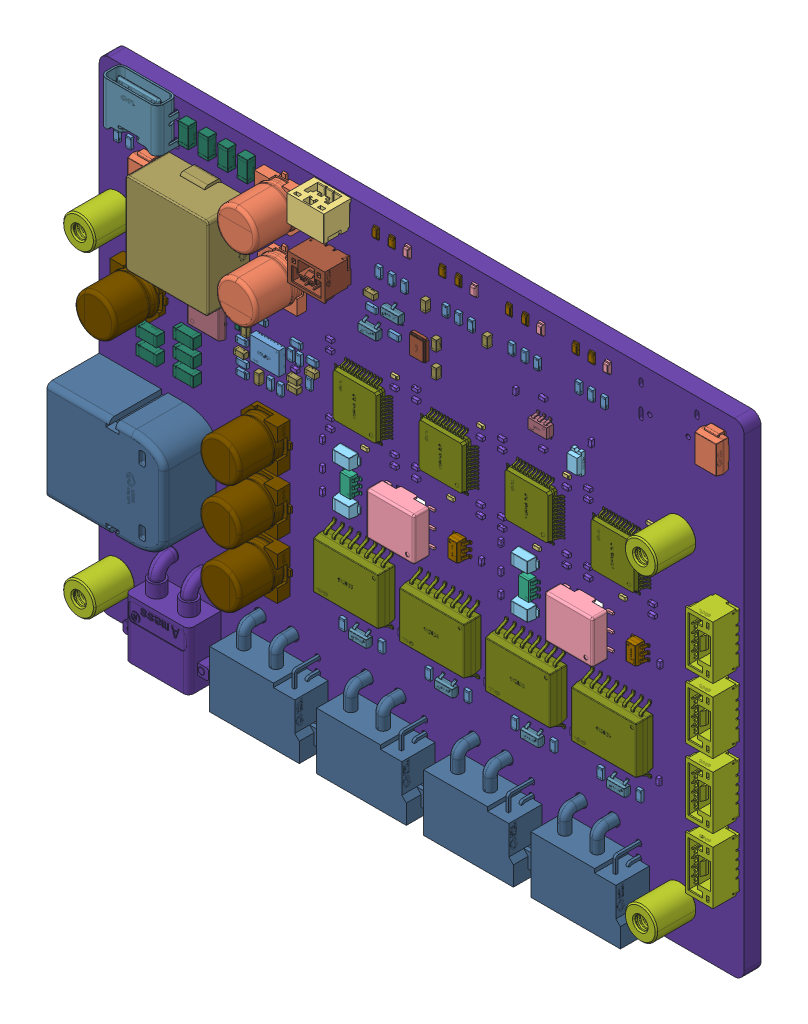
SolidWorks assembly 三合一(1), configuration 默认. Lengths in mm. (continued)
Components (placement in the parent): (continued)
- 三合一(1).step-1: 三合一(1).step [默认] at origin size (99.98 75.08 11.76) (continued)
  - X3~CRYSTAL-SMD_4P-L3.2-W2.5-BL~CRYSTAL-SMD_4P-L3.2-W2.5-BL~Huq4.step-1: X3~CRYSTAL-SMD_4P-L3.2-W2.5-BL~CRYSTAL-SMD_4P-L3.2-W2.5-BL~Huq4.step [默认] at (-11.176 22.9235 2.6301) x (0 -1 0) z (0 0 1) size (3.2 2.5 0.7)
    - CRYSTAL-SMD_4P-L3.2-W2.5-BL~CRYSTAL-SMD_4P-L3.2-W2.5-BL~nuzN.step-1: CRYSTAL-SMD_4P-L3.2-W2.5-BL~CRYSTAL-SMD_4P-L3.2-W2.5-BL~nuzN.step [默认] at origin size (3.2 2.5 0.7)
  - C143~C0603~C0603_L1.6-W0.8-H0.8~8vyH.step-1: C143~C0603~C0603_L1.6-W0.8-H0.8~8vyH.step [默认] at (-18.516 26.4431 3.0301) size (1.6 0.8 0.8)
    - C0603~C0603_L1.6-W0.8-H0.8~0uWZ.step-1: C0603~C0603_L1.6-W0.8-H0.8~0uWZ.step [默认] at origin size (1.6 0.8 0.8)
  - C141~C0603~C0603_L1.6-W0.8-H0.8~goz1.step-1: C141~C0603~C0603_L1.6-W0.8-H0.8~goz1.step [默认] at (-8.382 21.0424 3.0301) x (0 1 0) z (0 0 1) size (1.6 0.8 0.8)
    - C0603~C0603_L1.6-W0.8-H0.8~0uWZ.step-1: C0603~C0603_L1.6-W0.8-H0.8~0uWZ.step [默认] at origin size (1.6 0.8 0.8)
  - C142~C0603~C0603_L1.6-W0.8-H0.8~5pQK.step-1: C142~C0603~C0603_L1.6-W0.8-H0.8~5pQK.step [默认] at (-8.382 24.8046 3.0301) x (0 -1 0) z (0 0 1) size (1.6 0.8 0.8)
    - C0603~C0603_L1.6-W0.8-H0.8~0uWZ.step-1: C0603~C0603_L1.6-W0.8-H0.8~0uWZ.step [默认] at origin size (1.6 0.8 0.8)
  - C139~C0603~C0603_L1.6-W0.8-H0.8~dp7c.step-1: C139~C0603~C0603_L1.6-W0.8-H0.8~dp7c.step [默认] at (-10.0359 29.2101 3.0301) x (0 1 0) z (0 0 1) size (1.6 0.8 0.8)
    - C0603~C0603_L1.6-W0.8-H0.8~0uWZ.step-1: C0603~C0603_L1.6-W0.8-H0.8~0uWZ.step [默认] at origin size (1.6 0.8 0.8)
  - C140~C0603~C0603_L1.6-W0.8-H0.8~3sRw.step-1: C140~C0603~C0603_L1.6-W0.8-H0.8~3sRw.step [默认] at (-0.482 29.2101 3.0301) x (0 1 0) z (0 0 1) size (1.6 0.8 0.8)
    - C0603~C0603_L1.6-W0.8-H0.8~0uWZ.step-1: C0603~C0603_L1.6-W0.8-H0.8~0uWZ.step [默认] at origin size (1.6 0.8 0.8)
  - C3~C0402~C0603_L1.6-W0.8-H0.8~DXB2.step-1: C3~C0402~C0603_L1.6-W0.8-H0.8~DXB2.step [默认] at (-30.4075 7.8146 3.0301) x (-1 0 0) z (0 0 1) size (1.6 0.8 0.8)
    - C0603~C0603_L1.6-W0.8-H0.8~0uWZ.step-1: C0603~C0603_L1.6-W0.8-H0.8~0uWZ.step [默认] at origin size (1.6 0.8 0.8)
  - C4~C0402~C0603_L1.6-W0.8-H0.8~lKWs.step-1: C4~C0402~C0603_L1.6-W0.8-H0.8~lKWs.step [默认] at (-35.8689 6.5373 3.0301) x (0 1 0) z (0 0 1) size (1.6 0.8 0.8)
    - C0603~C0603_L1.6-W0.8-H0.8~0uWZ.step-1: C0603~C0603_L1.6-W0.8-H0.8~0uWZ.step [默认] at origin size (1.6 0.8 0.8)
  - C5~C0402~C0603_L1.6-W0.8-H0.8~kbQX.step-1: C5~C0402~C0603_L1.6-W0.8-H0.8~kbQX.step [默认] at (-30.4075 9.0339 3.0301) x (-1 0 0) z (0 0 1) size (1.6 0.8 0.8)
    - C0603~C0603_L1.6-W0.8-H0.8~0uWZ.step-1: C0603~C0603_L1.6-W0.8-H0.8~0uWZ.step [默认] at origin size (1.6 0.8 0.8)
  - C6~C0402~C0603_L1.6-W0.8-H0.8~siWF.step-1: C6~C0402~C0603_L1.6-W0.8-H0.8~siWF.step [默认] at (-27.6478 11.2673 3.0301) size (1.6 0.8 0.8)
    - C0603~C0603_L1.6-W0.8-H0.8~0uWZ.step-1: C0603~C0603_L1.6-W0.8-H0.8~0uWZ.step [默认] at origin size (1.6 0.8 0.8)
  - C7~C0402~C0603_L1.6-W0.8-H0.8~Gngn.step-1: C7~C0402~C0603_L1.6-W0.8-H0.8~Gngn.step [默认] at (-37.8461 11.938 3.0301) x (0 -1 0) z (0 0 1) size (1.6 0.8 0.8)
    - C0603~C0603_L1.6-W0.8-H0.8~0uWZ.step-1: C0603~C0603_L1.6-W0.8-H0.8~0uWZ.step [默认] at origin size (1.6 0.8 0.8)
  - C8~C0402~C0603_L1.6-W0.8-H0.8~xPmg.step-1: C8~C0402~C0603_L1.6-W0.8-H0.8~xPmg.step [默认] at (-47.1845 12.2066 -0.4) x (0 1 0) z (0 0 -1) size (1.6 0.8 0.8)
    - C0603~C0603_L1.6-W0.8-H0.8~0uWZ.step-1: C0603~C0603_L1.6-W0.8-H0.8~0uWZ.step [默认] at origin size (1.6 0.8 0.8)
  - C9~C0402~C0603_L1.6-W0.8-H0.8~Sl4T.step-1: C9~C0402~C0603_L1.6-W0.8-H0.8~Sl4T.step [默认] at (-38.6381 8.4432 3.0301) size (1.6 0.8 0.8)
    - C0603~C0603_L1.6-W0.8-H0.8~0uWZ.step-1: C0603~C0603_L1.6-W0.8-H0.8~0uWZ.step [默认] at origin size (1.6 0.8 0.8)
  - U117~SOT-23-5_L2.9-W1.6-P0.95-LS2.8-BL~SOT-23-5_L2.9-W1.6-P0.95-LS2.8-BL~xtDB.step-1: U117~SOT-23-5_L2.9-W1.6-P0.95-LS2.8-BL~SOT-23-5_L2.9-W1.6-P0.95-LS2.8-BL~xtDB.step [默认] at (8.032 21.986 3.3801) x (-1 0 0) z (0 0 1) size (2.92 2.8 1.15)
    - SOT-23-5_L2.9-W1.6-P0.95-LS2.8-BL~SOT-23-5_L2.9-W1.6-P0.95-LS2.8-BL~GdKc.step-1: SOT-23-5_L2.9-W1.6-P0.95-LS2.8-BL~SOT-23-5_L2.9-W1.6-P0.95-LS2.8-BL~GdKc.step [默认] at origin size (2.92 2.8 1.15)
  - Q3~SOT-23-3_L2.9-W1.3-P1.90-LS2.4-BR~SOT-23-3P_L2.9-W1.3-H1.0-LS2.4-P0.95~UPIG.step-1: Q3~SOT-23-3_L2.9-W1.3-P1.90-LS2.4-BR~SOT-23-3P_L2.9-W1.3-H1.0-LS2.4-P0.95~UPIG.step [默认] at (-18.516 21.6171 2.5794) x (0 -1 0) z (0 0 1) size (2.5 2.89 1.05)
    - SOT-23-3_L2.9-W1.3-P1.90-LS2.4-BR~SOT-23-3P_L2.9-W1.3-H1.0-LS2.4-P0.95~rVWb.step-1: SOT-23-3_L2.9-W1.3-P1.90-LS2.4-BR~SOT-23-3P_L2.9-W1.3-H1.0-LS2.4-P0.95~rVWb.step [默认] at origin size (2.5 2.89 1.05)
  - D11~SOT-23-3_L2.9-W1.3-P1.90-LS2.4-BR~SOT-23-3P_L2.9-W1.3-H1.0-LS2.4-P0.95~v811.step-1: D11~SOT-23-3_L2.9-W1.3-P1.90-LS2.4-BR~SOT-23-3P_L2.9-W1.3-H1.0-LS2.4-P0.95~v811.step [默认] at (-20 -20.3843 2.5794) x (0 -1 0) z (0 0 1) size (2.5 2.89 1.05)
    - SOT-23-3_L2.9-W1.3-P1.90-LS2.4-BR~SOT-23-3P_L2.9-W1.3-H1.0-LS2.4-P0.95~rVWb.step-1: SOT-23-3_L2.9-W1.3-P1.90-LS2.4-BR~SOT-23-3P_L2.9-W1.3-H1.0-LS2.4-P0.95~rVWb.step [默认] at origin size (2.5 2.89 1.05)
  - Q4~SOT-23-3_L2.9-W1.3-P1.90-LS2.4-BR~SOT-23-3P_L2.9-W1.3-H1.0-LS2.4-P0.95~4c30.step-1: Q4~SOT-23-3_L2.9-W1.3-P1.90-LS2.4-BR~SOT-23-3P_L2.9-W1.3-H1.0-LS2.4-P0.95~4c30.step [默认] at (-15.016 25.527 2.5794) x (0 1 0) z (0 0 1) size (2.5 2.89 1.05)
    - SOT-23-3_L2.9-W1.3-P1.90-LS2.4-BR~SOT-23-3P_L2.9-W1.3-H1.0-LS2.4-P0.95~rVWb.step-1: SOT-23-3_L2.9-W1.3-P1.90-LS2.4-BR~SOT-23-3P_L2.9-W1.3-H1.0-LS2.4-P0.95~rVWb.step [默认] at origin size (2.5 2.89 1.05)
  - D12~SOT-23-3_L2.9-W1.3-P1.90-LS2.4-BR~SOT-23-3P_L2.9-W1.3-H1.0-LS2.4-P0.95~vKNW.step-1: D12~SOT-23-3_L2.9-W1.3-P1.90-LS2.4-BR~SOT-23-3P_L2.9-W1.3-H1.0-LS2.4-P0.95~vKNW.step [默认] at (-6.6667 -20.3843 2.5794) x (0 -1 0) z (0 0 1) size (2.5 2.89 1.05)
    - SOT-23-3_L2.9-W1.3-P1.90-LS2.4-BR~SOT-23-3P_L2.9-W1.3-H1.0-LS2.4-P0.95~rVWb.step-1: SOT-23-3_L2.9-W1.3-P1.90-LS2.4-BR~SOT-23-3P_L2.9-W1.3-H1.0-LS2.4-P0.95~rVWb.step [默认] at origin size (2.5 2.89 1.05)
  - D13~SOT-23-3_L2.9-W1.3-P1.90-LS2.4-BR~SOT-23-3P_L2.9-W1.3-H1.0-LS2.4-P0.95~TBOq.step-1: D13~SOT-23-3_L2.9-W1.3-P1.90-LS2.4-BR~SOT-23-3P_L2.9-W1.3-H1.0-LS2.4-P0.95~TBOq.step [默认] at (6.6667 -20.3843 2.5794) x (0 -1 0) z (0 0 1) size (2.5 2.89 1.05)
    - SOT-23-3_L2.9-W1.3-P1.90-LS2.4-BR~SOT-23-3P_L2.9-W1.3-H1.0-LS2.4-P0.95~rVWb.step-1: SOT-23-3_L2.9-W1.3-P1.90-LS2.4-BR~SOT-23-3P_L2.9-W1.3-H1.0-LS2.4-P0.95~rVWb.step [默认] at origin size (2.5 2.89 1.05)
  - D14~SOT-23-3_L2.9-W1.3-P1.90-LS2.4-BR~SOT-23-3P_L2.9-W1.3-H1.0-LS2.4-P0.95~BLMC.step-1: D14~SOT-23-3_L2.9-W1.3-P1.90-LS2.4-BR~SOT-23-3P_L2.9-W1.3-H1.0-LS2.4-P0.95~BLMC.step [默认] at (20.0001 -20.3843 2.5794) x (0 -1 0) z (0 0 1) size (2.5 2.89 1.05)
    - SOT-23-3_L2.9-W1.3-P1.90-LS2.4-BR~SOT-23-3P_L2.9-W1.3-H1.0-LS2.4-P0.95~rVWb.step-1: SOT-23-3_L2.9-W1.3-P1.90-LS2.4-BR~SOT-23-3P_L2.9-W1.3-H1.0-LS2.4-P0.95~rVWb.step [默认] at origin size (2.5 2.89 1.05)
  - D2~SOD-523F_L1.2-W0.8-LS1.7-RD~SOD-523F_L1.2-W0.8-H0.6-LS1.6~9aiK.step-1: D2~SOD-523F_L1.2-W0.8-LS1.7-RD~SOD-523F_L1.2-W0.8-H0.6-LS1.6~9aiK.step [默认] at (-39.0687 11.945 2.6301) x (0 1 0) z (0 0 1) size (1.6 0.8 0.61)
    - SOD-523F_L1.2-W0.8-LS1.7-RD~SOD-523F_L1.2-W0.8-H0.6-LS1.6~e6mV.step-1: SOD-523F_L1.2-W0.8-LS1.7-RD~SOD-523F_L1.2-W0.8-H0.6-LS1.6~e6mV.step [默认] at origin size (1.6 0.8 0.61)
  - U25~SOIC-16_L10.3-W7.5-P1.27-LS10.3-BL~SOIC-16_L10.3-W7.5-H2.7-LS10.3-P1.27~kk9U.step-1: U25~SOIC-16_L10.3-W7.5-P1.27-LS10.3-BL~SOIC-16_L10.3-W7.5-H2.7-LS10.3-P1.27~kk9U.step [默认] at (-20 -12 2.6795) x (-1 0 0) z (0 0 1) size (10.3 10.41 2.85)
    - SOIC-16_L10.3-W7.5-P1.27-LS10.3-BL~SOIC-16_L10.3-W7.5-H2.7-LS10.3-P1.27~Lkft.step-1: SOIC-16_L10.3-W7.5-P1.27-LS10.3-BL~SOIC-16_L10.3-W7.5-H2.7-LS10.3-P1.27~Lkft.step [默认] at origin size (10.3 10.41 2.85)
  - U111~SOIC-16_L10.3-W7.5-P1.27-LS10.3-BL~SOIC-16_L10.3-W7.5-H2.7-LS10.3-P1.27~qvoO.step-1: U111~SOIC-16_L10.3-W7.5-P1.27-LS10.3-BL~SOIC-16_L10.3-W7.5-H2.7-LS10.3-P1.27~qvoO.step [默认] at (-6.6667 -12 2.6795) x (-1 0 0) z (0 0 1) size (10.3 10.41 2.85)
    - SOIC-16_L10.3-W7.5-P1.27-LS10.3-BL~SOIC-16_L10.3-W7.5-H2.7-LS10.3-P1.27~Lkft.step-1: SOIC-16_L10.3-W7.5-P1.27-LS10.3-BL~SOIC-16_L10.3-W7.5-H2.7-LS10.3-P1.27~Lkft.step [默认] at origin size (10.3 10.41 2.85)
  - U113~SOIC-16_L10.3-W7.5-P1.27-LS10.3-BL~SOIC-16_L10.3-W7.5-H2.7-LS10.3-P1.27~DOeF.step-1: U113~SOIC-16_L10.3-W7.5-P1.27-LS10.3-BL~SOIC-16_L10.3-W7.5-H2.7-LS10.3-P1.27~DOeF.step [默认] at (6.6667 -12 2.6795) x (-1 0 0) z (0 0 1) size (10.3 10.41 2.85)
    - SOIC-16_L10.3-W7.5-P1.27-LS10.3-BL~SOIC-16_L10.3-W7.5-H2.7-LS10.3-P1.27~Lkft.step-1: SOIC-16_L10.3-W7.5-P1.27-LS10.3-BL~SOIC-16_L10.3-W7.5-H2.7-LS10.3-P1.27~Lkft.step [默认] at origin size (10.3 10.41 2.85)
  - U115~SOIC-16_L10.3-W7.5-P1.27-LS10.3-BL~SOIC-16_L10.3-W7.5-H2.7-LS10.3-P1.27~A0C9.step-1: U115~SOIC-16_L10.3-W7.5-P1.27-LS10.3-BL~SOIC-16_L10.3-W7.5-H2.7-LS10.3-P1.27~A0C9.step [默认] at (20.0001 -12 2.6795) x (-1 0 0) z (0 0 1) size (10.3 10.41 2.85)
    - SOIC-16_L10.3-W7.5-P1.27-LS10.3-BL~SOIC-16_L10.3-W7.5-H2.7-LS10.3-P1.27~Lkft.step-1: SOIC-16_L10.3-W7.5-P1.27-LS10.3-BL~SOIC-16_L10.3-W7.5-H2.7-LS10.3-P1.27~Lkft.step [默认] at origin size (10.3 10.41 2.85)
  - CN3~CONN-TH_XT30PW-M~CONN-TH_XT30PW-M~k8yd.step-1: CN3~CONN-TH_XT30PW-M~CONN-TH_XT30PW-M~k8yd.step [默认] at (-47.1172 -32.6901 2.6301) size (13.3 13.95 7.01)
    - CONN-TH_XT30PW-M~CONN-TH_XT30PW-M~GxAZ.step-1: CONN-TH_XT30PW-M~CONN-TH_XT30PW-M~GxAZ.step [默认] at origin size (13.3 13.95 7.01)
  - C1~CAP-SMD_BD6.3-L6.6-W6.6-LS7.3-FD-H7.7~CAP-SMD_BD6.3-L6.6-W6.6-LS7.3-FD-H7.7~O7oJ.step-1: C1~CAP-SMD_BD6.3-L6.6-W6.6-LS7.3-FD-H7.7~CAP-SMD_BD6.3-L6.6-W6.6-LS7.3-FD-H7.7~O7oJ.step [默认] at (-34.7324 -0.4769 2.6301) size (7.3 6.6 7.7)
    - CAP-SMD_BD6.3-L6.6-W6.6-LS7.3-FD-H7.7~CAP-SMD_BD6.3-L6.6-W6.6-LS7.3-FD-H7.7~e4JW.step-1: CAP-SMD_BD6.3-L6.6-W6.6-LS7.3-FD-H7.7~CAP-SMD_BD6.3-L6.6-W6.6-LS7.3-FD-H7.7~e4JW.step [默认] at origin size (7.3 6.6 7.7)
  - C19~CAP-SMD_BD6.3-L6.6-W6.6-LS7.3-FD-H7.7~CAP-SMD_BD6.3-L6.6-W6.6-LS7.3-FD-H7.7~UGRS.step-1: C19~CAP-SMD_BD6.3-L6.6-W6.6-LS7.3-FD-H7.7~CAP-SMD_BD6.3-L6.6-W6.6-LS7.3-FD-H7.7~UGRS.step [默认] at (-54.0561 9.265 2.6301) x (-1 0 0) z (0 0 1) size (7.3 6.6 7.7)
    - CAP-SMD_BD6.3-L6.6-W6.6-LS7.3-FD-H7.7~CAP-SMD_BD6.3-L6.6-W6.6-LS7.3-FD-H7.7~e4JW.step-1: CAP-SMD_BD6.3-L6.6-W6.6-LS7.3-FD-H7.7~CAP-SMD_BD6.3-L6.6-W6.6-LS7.3-FD-H7.7~e4JW.step [默认] at origin size (7.3 6.6 7.7)
  - C22~CAP-SMD_BD6.3-L6.6-W6.6-LS7.3-FD-H7.7~CAP-SMD_BD6.3-L6.6-W6.6-LS7.3-FD-H7.7~cbLl.step-1: C22~CAP-SMD_BD6.3-L6.6-W6.6-LS7.3-FD-H7.7~CAP-SMD_BD6.3-L6.6-W6.6-LS7.3-FD-H7.7~cbLl.step [默认] at (-34.7324 -9.0035 2.6301) size (7.3 6.6 7.7)
    - CAP-SMD_BD6.3-L6.6-W6.6-LS7.3-FD-H7.7~CAP-SMD_BD6.3-L6.6-W6.6-LS7.3-FD-H7.7~e4JW.step-1: CAP-SMD_BD6.3-L6.6-W6.6-LS7.3-FD-H7.7~CAP-SMD_BD6.3-L6.6-W6.6-LS7.3-FD-H7.7~e4JW.step [默认] at origin size (7.3 6.6 7.7)
  - C23~CAP-SMD_BD6.3-L6.6-W6.6-LS7.3-FD-H7.7~CAP-SMD_BD6.3-L6.6-W6.6-LS7.3-FD-H7.7~3RQV.step-1: C23~CAP-SMD_BD6.3-L6.6-W6.6-LS7.3-FD-H7.7~CAP-SMD_BD6.3-L6.6-W6.6-LS7.3-FD-H7.7~3RQV.step [默认] at (-34.7324 -17.5302 2.6301) size (7.3 6.6 7.7)
    - CAP-SMD_BD6.3-L6.6-W6.6-LS7.3-FD-H7.7~CAP-SMD_BD6.3-L6.6-W6.6-LS7.3-FD-H7.7~e4JW.step-1: CAP-SMD_BD6.3-L6.6-W6.6-LS7.3-FD-H7.7~CAP-SMD_BD6.3-L6.6-W6.6-LS7.3-FD-H7.7~e4JW.step [默认] at origin size (7.3 6.6 7.7)
  - U1~VQFN-20_L4.5-W3.5-P0.50-BL-EP~VQFN-20_L4.5-W3.5-H1.0-P0.50-BL-EP~KmcK.step-1: U1~VQFN-20_L4.5-W3.5-P0.50-BL-EP~VQFN-20_L4.5-W3.5-H1.0-P0.50-BL-EP~KmcK.step [默认] at (-34.4421 10.4503 2.6301) x (-1 0 0) z (0 0 1) size (4.52 3.52 1.02)
    - VQFN-20_L4.5-W3.5-P0.50-BL-EP~VQFN-20_L4.5-W3.5-H1.0-P0.50-BL-EP~r6FV.step-1: VQFN-20_L4.5-W3.5-P0.50-BL-EP~VQFN-20_L4.5-W3.5-H1.0-P0.50-BL-EP~r6FV.step [默认] at origin size (4.52 3.52 1.02)
  - C14~CAP-SMD_BD6.3-L6.6-W6.6-FD~CAP-SMD_BD6.3-L6.6-W6.6-FD~sTGZ.step-1: C14~CAP-SMD_BD6.3-L6.6-W6.6-FD~CAP-SMD_BD6.3-L6.6-W6.6-FD~sTGZ.step [默认] at (-32.1308 22.096 2.6801) x (0 1 0) z (0 0 1) size (7.8 6.6 7.75)
    - CAP-SMD_BD6.3-L6.6-W6.6-FD~CAP-SMD_BD6.3-L6.6-W6.6-FD~IJAE.step-1: CAP-SMD_BD6.3-L6.6-W6.6-FD~CAP-SMD_BD6.3-L6.6-W6.6-FD~IJAE.step [默认] at origin size (7.8 6.6 7.75)
  - C20~CAP-SMD_BD6.3-L6.6-W6.6-FD~CAP-SMD_BD6.3-L6.6-W6.6-FD~PgOv.step-1: C20~CAP-SMD_BD6.3-L6.6-W6.6-FD~CAP-SMD_BD6.3-L6.6-W6.6-FD~PgOv.step [默认] at (-32.1303 31.8537 2.6801) x (0 -1 0) z (0 0 1) size (7.8 6.6 7.75)
    - CAP-SMD_BD6.3-L6.6-W6.6-FD~CAP-SMD_BD6.3-L6.6-W6.6-FD~IJAE.step-1: CAP-SMD_BD6.3-L6.6-W6.6-FD~CAP-SMD_BD6.3-L6.6-W6.6-FD~IJAE.step [默认] at origin size (7.8 6.6 7.75)
  - CN1~CONN-TH_2P-P1.25_XUNPU_WAFER-GH1.25-2PWB~CONN-TH_2P-P1.25_XUNPU_WAFER-GH1.25-2PWB~8efc.step-1: CN1~CONN-TH_2P-P1.25_XUNPU_WAFER-GH1.25-2PWB~CONN-TH_2P-P1.25_XUNPU_WAFER-GH1.25-2PWB~8efc.step [默认] at (-24.7295 35.3981 6.9801) x (-1 0 0) z (0 0 1) size (5.76 5 4.35)
    - CONN-TH_2P-P1.25_XUNPU_WAFER-GH1.25-2PWB~CONN-TH_2P-P1.25_XUNPU_WAFER-GH1.25-2PWB~vxTZ.step-1: CONN-TH_2P-P1.25_XUNPU_WAFER-GH1.25-2PWB~CONN-TH_2P-P1.25_XUNPU_WAFER-GH1.25-2PWB~vxTZ.step [默认] at origin size (5.76 5 4.35)
  - T5~XFMR-SMD_L7.5-W6.7-P2.54-LS7.7-BL~XFMR-SMD_L7.5-W6.7-P2.54-LS7.7-BL~cbkL.step-1: T5~XFMR-SMD_L7.5-W6.7-P2.54-LS7.7-BL~XFMR-SMD_L7.5-W6.7-P2.54-LS7.7-BL~cbkL.step [默认] at (15 -0.508 2.9301) x (0 1 0) z (0 0 1) size (6.65 7.7 3.3)
    - XFMR-SMD_L7.5-W6.7-P2.54-LS7.7-BL~XFMR-SMD_L7.5-W6.7-P2.54-LS7.7-BL~W4hX.step-1: XFMR-SMD_L7.5-W6.7-P2.54-LS7.7-BL~XFMR-SMD_L7.5-W6.7-P2.54-LS7.7-BL~W4hX.step [默认] at origin size (6.65 7.7 3.3)
  - T6~XFMR-SMD_L7.5-W6.7-P2.54-LS7.7-BL~XFMR-SMD_L7.5-W6.7-P2.54-LS7.7-BL~mkAI.step-1: T6~XFMR-SMD_L7.5-W6.7-P2.54-LS7.7-BL~XFMR-SMD_L7.5-W6.7-P2.54-LS7.7-BL~mkAI.step [默认] at (-12.662 -0.508 2.9301) x (0 1 0) z (0 0 1) size (6.65 7.7 3.3)
    - XFMR-SMD_L7.5-W6.7-P2.54-LS7.7-BL~XFMR-SMD_L7.5-W6.7-P2.54-LS7.7-BL~W4hX.step-1: XFMR-SMD_L7.5-W6.7-P2.54-LS7.7-BL~XFMR-SMD_L7.5-W6.7-P2.54-LS7.7-BL~W4hX.step [默认] at origin size (6.65 7.7 3.3)
  - LED29~LED0603_RED~LED-0603_R~n785.step-1: LED29~LED0603_RED~LED-0603_R~n785.step [默认] at (13.462 19.939 2.6321) x (0 -1 0) z (0 0 1) size (3.22 1.61 1.21)
    - LED0603_RED~LED-0603_R~z5gK.step-1: LED0603_RED~LED-0603_R~z5gK.step [默认] at origin size (3.22 1.61 1.21)
  - D1~TSDSON-8-FL_L3.3-W3.3-P0.65-BL~TSDSON-8-FL_L3.3-W3.3-P0.65-BL~Tfhm.step-1: D1~TSDSON-8-FL_L3.3-W3.3-P0.65-BL~TSDSON-8-FL_L3.3-W3.3-P0.65-BL~Tfhm.step [默认] at (-44.2452 10.5114 -0.02) x (-1 0 0) z (0 0 -1) size (3.3 3.3 1.02)
    - TSDSON-8-FL_L3.3-W3.3-P0.65-BL~TSDSON-8-FL_L3.3-W3.3-P0.65-BL~zgzj.step-1: TSDSON-8-FL_L3.3-W3.3-P0.65-BL~TSDSON-8-FL_L3.3-W3.3-P0.65-BL~zgzj.step [默认] at origin size (3.3 3.3 1.02)
  - U17~CONN-SMD_4P-P1.25_XUNPU_WAFER-GH1.25-4PLB~CONN-TH_4P-P1.25_XUNPU_WAFER-GH1.25-4PLB~TT0J.step-1: U17~CONN-SMD_4P-P1.25_XUNPU_WAFER-GH1.25-4PLB~CONN-TH_4P-P1.25_XUNPU_WAFER-GH1.25-4PLB~TT0J.step [默认] at (35.835 -11.6416 2.7801) x (0 -1 0) z (0 0 1) size (8.25 4.95 4.2)
    - CONN-SMD_4P-P1.25_XUNPU_WAFER-GH1.25-4PLB~CONN-TH_4P-P1.25_XUNPU_WAFER-GH1.25-4PLB~FJiB.step-1: CONN-SMD_4P-P1.25_XUNPU_WAFER-GH1.25-4PLB~CONN-TH_4P-P1.25_XUNPU_WAFER-GH1.25-4PLB~FJiB.step [默认] at origin size (8.25 4.95 4.2)
  - U18~CONN-SMD_4P-P1.25_XUNPU_WAFER-GH1.25-4PLB~CONN-TH_4P-P1.25_XUNPU_WAFER-GH1.25-4PLB~1LlB.step-1: U18~CONN-SMD_4P-P1.25_XUNPU_WAFER-GH1.25-4PLB~CONN-TH_4P-P1.25_XUNPU_WAFER-GH1.25-4PLB~1LlB.step [默认] at (35.835 -1.5663 2.7801) x (0 -1 0) z (0 0 1) size (8.25 4.95 4.2)
    - CONN-SMD_4P-P1.25_XUNPU_WAFER-GH1.25-4PLB~CONN-TH_4P-P1.25_XUNPU_WAFER-GH1.25-4PLB~FJiB.step-1: CONN-SMD_4P-P1.25_XUNPU_WAFER-GH1.25-4PLB~CONN-TH_4P-P1.25_XUNPU_WAFER-GH1.25-4PLB~FJiB.step [默认] at origin size (8.25 4.95 4.2)
  - U19~CONN-SMD_4P-P1.25_XUNPU_WAFER-GH1.25-4PLB~CONN-TH_4P-P1.25_XUNPU_WAFER-GH1.25-4PLB~ZuVo.step-1: U19~CONN-SMD_4P-P1.25_XUNPU_WAFER-GH1.25-4PLB~CONN-TH_4P-P1.25_XUNPU_WAFER-GH1.25-4PLB~ZuVo.step [默认] at (35.835 8.5091 2.7801) x (0 -1 0) z (0 0 1) size (8.25 4.95 4.2)
    - CONN-SMD_4P-P1.25_XUNPU_WAFER-GH1.25-4PLB~CONN-TH_4P-P1.25_XUNPU_WAFER-GH1.25-4PLB~FJiB.step-1: CONN-SMD_4P-P1.25_XUNPU_WAFER-GH1.25-4PLB~CONN-TH_4P-P1.25_XUNPU_WAFER-GH1.25-4PLB~FJiB.step [默认] at origin size (8.25 4.95 4.2)
  - U16~CONN-SMD_4P-P1.25_XUNPU_WAFER-GH1.25-4PLB~CONN-TH_4P-P1.25_XUNPU_WAFER-GH1.25-4PLB~uRby.step-1: U16~CONN-SMD_4P-P1.25_XUNPU_WAFER-GH1.25-4PLB~CONN-TH_4P-P1.25_XUNPU_WAFER-GH1.25-4PLB~uRby.step [默认] at (35.835 -21.717 2.7801) x (0 -1 0) z (0 0 1) size (8.25 4.95 4.2)
    - CONN-SMD_4P-P1.25_XUNPU_WAFER-GH1.25-4PLB~CONN-TH_4P-P1.25_XUNPU_WAFER-GH1.25-4PLB~FJiB.step-1: CONN-SMD_4P-P1.25_XUNPU_WAFER-GH1.25-4PLB~CONN-TH_4P-P1.25_XUNPU_WAFER-GH1.25-4PLB~FJiB.step [默认] at origin size (8.25 4.95 4.2)
  - Q2~DFN-8_L3.3-W3.3-P0.65-BL-3~DFN-8_L3.3-W3.3-P0.65-BL-3~YrRQ.step-1: Q2~DFN-8_L3.3-W3.3-P0.65-BL-3~DFN-8_L3.3-W3.3-P0.65-BL-3~YrRQ.step [默认] at (-48.6411 14.478 2.6401) x (0 1 0) z (0 0 1) size (3.3 3.32 0.77)
    - DFN-8_L3.3-W3.3-P0.65-BL-3~DFN-8_L3.3-W3.3-P0.65-BL-3~jhzz.step-1: DFN-8_L3.3-W3.3-P0.65-BL-3~DFN-8_L3.3-W3.3-P0.65-BL-3~jhzz.step [默认] at origin size (3.3 3.32 0.77)
  - U106~SOT-23-6_L2.9-W1.6-P0.95-LS2.8-BR~SOT-23-6_L2.9-W1.6-H1.5-LS2.8-P0.95~IPVb.step-1: U106~SOT-23-6_L2.9-W1.6-P0.95-LS2.8-BR~SOT-23-6_L2.9-W1.6-H1.5-LS2.8-P0.95~IPVb.step [默认] at (23 -0.5079 2.679) size (2.81 2.9 1.65)
    - SOT-23-6_L2.9-W1.6-P0.95-LS2.8-BR~SOT-23-6_L2.9-W1.6-H1.5-LS2.8-P0.95~IDnD.step-1: SOT-23-6_L2.9-W1.6-P0.95-LS2.8-BR~SOT-23-6_L2.9-W1.6-H1.5-LS2.8-P0.95~IDnD.step [默认] at origin size (2.81 2.9 1.65)
  - U29~SOT-23-6_L2.9-W1.6-P0.95-LS2.8-BR~SOT-23-6_L2.9-W1.6-H1.5-LS2.8-P0.95~uDfg.step-1: U29~SOT-23-6_L2.9-W1.6-P0.95-LS2.8-BR~SOT-23-6_L2.9-W1.6-H1.5-LS2.8-P0.95~uDfg.step [默认] at (-4.662 -0.5079 2.679) size (2.81 2.9 1.65)
    - SOT-23-6_L2.9-W1.6-P0.95-LS2.8-BR~SOT-23-6_L2.9-W1.6-H1.5-LS2.8-P0.95~IDnD.step-1: SOT-23-6_L2.9-W1.6-P0.95-LS2.8-BR~SOT-23-6_L2.9-W1.6-H1.5-LS2.8-P0.95~IDnD.step [默认] at origin size (2.81 2.9 1.65)
  - CN2~CONN-TH_XT60PW-M~CONN-TH_XT60PW-M~LJHb.step-1: CN2~CONN-TH_XT60PW-M~CONN-TH_XT60PW-M~LJHb.step [默认] at (-51.9869 -10.7515 2.6301) size (18.18 15.59 11.11)
    - CONN-TH_XT60PW-M~CONN-TH_XT60PW-M~7bWj.step-1: CONN-TH_XT60PW-M~CONN-TH_XT60PW-M~7bWj.step [默认] at origin size (18.18 15.59 11.11)
  - CN4~CONN-TH_2P-P1.25_XUNPU_WAFER-GH1.25-2PLB~CONN-TH_2P-P1.25_XUNPU_WAFER-GH1.25-2PLB~jJN7.step-1: CN4~CONN-TH_2P-P1.25_XUNPU_WAFER-GH1.25-2PLB~CONN-TH_2P-P1.25_XUNPU_WAFER-GH1.25-2PLB~jJN7.step [默认] at (-24.7395 27.0787 2.7801) size (5.76 4.95 4.2)
    - CONN-TH_2P-P1.25_XUNPU_WAFER-GH1.25-2PLB~CONN-TH_2P-P1.25_XUNPU_WAFER-GH1.25-2PLB~ErAg.step-1: CONN-TH_2P-P1.25_XUNPU_WAFER-GH1.25-2PLB~CONN-TH_2P-P1.25_XUNPU_WAFER-GH1.25-2PLB~ErAg.step [默认] at origin size (5.76 4.95 4.2)
  - L1~IND-SMD_L12.8-W12.8-LS13.8_CYA1265~IND-SMD_L12.8-W12.8-LS13.8_CYA1265~jbXl.step-1: L1~IND-SMD_L12.8-W12.8-LS13.8_CYA1265~IND-SMD_L12.8-W12.8-LS13.8_CYA1265~jbXl.step [默认] at (-44.0741 23.114 2.7301) x (0 1 0) z (0 0 1) size (13.8 12.81 6.5)
    - IND-SMD_L12.8-W12.8-LS13.8_CYA1265~IND-SMD_L12.8-W12.8-LS13.8_CYA1265~kuI6.step-1: IND-SMD_L12.8-W12.8-LS13.8_CYA1265~IND-SMD_L12.8-W12.8-LS13.8_CYA1265~kuI6.step [默认] at origin size (13.8 12.81 6.5)
  - Q1~DFN-8_L5.9-W5.1-P1.27-LS6.1-BL-1~DFN-8_L5.9-W5.1-P1.27-LS6.1-BL-1~hMtS.step-1: Q1~DFN-8_L5.9-W5.1-P1.27-LS6.1-BL-1~DFN-8_L5.9-W5.1-P1.27-LS6.1-BL-1~hMtS.step [默认] at (-43.9287 11.6502 2.6301) size (5.33 6.16 1.06)
    - DFN-8_L5.9-W5.1-P1.27-LS6.1-BL-1~DFN-8_L5.9-W5.1-P1.27-LS6.1-BL-1~F0b2.step-1: DFN-8_L5.9-W5.1-P1.27-LS6.1-BL-1~DFN-8_L5.9-W5.1-P1.27-LS6.1-BL-1~F0b2.step [默认] at origin size (5.33 6.16 1.06)
  - USB11~TYPE-C-SMD_TYPE-C-6P~TYPE-C-SMD_6P-L8.9-W6.8-H3.2-P1.00~MEaq.step-1: USB11~TYPE-C-SMD_TYPE-C-6P~TYPE-C-SMD_6P-L8.9-W6.8-H3.2-P1.00~MEaq.step [默认] at (-53.3401 34.9933 2.5701) size (8.94 6.8 4.16)
    - TYPE-C-SMD_TYPE-C-6P~TYPE-C-SMD_6P-L8.9-W6.8-H3.2-P1.00~iyXO.step-1: TYPE-C-SMD_TYPE-C-6P~TYPE-C-SMD_6P-L8.9-W6.8-H3.2-P1.00~iyXO.step [默认] at origin size (8.94 6.8 4.16)
  - C18~C1206~C1206_L3.2-W1.6-H1.3~9jCj.step-1: C18~C1206~C1206_L3.2-W1.6-H1.3~9jCj.step [默认] at (-52.4563 4.1909 3.2801) size (3.2 1.6 1.3)
    - C1206~C1206_L3.2-W1.6-H1.3~cfxb.step-1: C1206~C1206_L3.2-W1.6-H1.3~cfxb.step [默认] at origin size (3.2 1.6 1.3)
  - C13~C1206~C1206_L3.2-W1.6-H1.3~WRU3.step-1: C13~C1206~C1206_L3.2-W1.6-H1.3~WRU3.step [默认] at (-37.568 34.0657 3.2801) x (0 -1 0) z (0 0 1) size (3.2 1.6 1.3)
    - C1206~C1206_L3.2-W1.6-H1.3~cfxb.step-1: C1206~C1206_L3.2-W1.6-H1.3~cfxb.step [默认] at origin size (3.2 1.6 1.3)
  - C11~C1206~C1206_L3.2-W1.6-H1.3~l9KQ.step-1: C11~C1206~C1206_L3.2-W1.6-H1.3~l9KQ.step [默认] at (-40.616 34.0657 3.2801) x (0 -1 0) z (0 0 1) size (3.2 1.6 1.3)
    - C1206~C1206_L3.2-W1.6-H1.3~cfxb.step-1: C1206~C1206_L3.2-W1.6-H1.3~cfxb.step [默认] at origin size (3.2 1.6 1.3)
  - C10~C1206~C1206_L3.2-W1.6-H1.3~Rkie.step-1: C10~C1206~C1206_L3.2-W1.6-H1.3~Rkie.step [默认] at (-43.664 34.0657 3.2801) x (0 -1 0) z (0 0 1) size (3.2 1.6 1.3)
    - C1206~C1206_L3.2-W1.6-H1.3~cfxb.step-1: C1206~C1206_L3.2-W1.6-H1.3~cfxb.step [默认] at origin size (3.2 1.6 1.3)
  - C12~C1206~C1206_L3.2-W1.6-H1.3~vEcB.step-1: C12~C1206~C1206_L3.2-W1.6-H1.3~vEcB.step [默认] at (-46.712 34.0657 3.2801) x (0 -1 0) z (0 0 1) size (3.2 1.6 1.3)
    - C1206~C1206_L3.2-W1.6-H1.3~cfxb.step-1: C1206~C1206_L3.2-W1.6-H1.3~cfxb.step [默认] at origin size (3.2 1.6 1.3)
  - C15~C1206~C1206_L3.2-W1.6-H1.3~8tLa.step-1: C15~C1206~C1206_L3.2-W1.6-H1.3~8tLa.step [默认] at (-46.7361 1.6509 3.2801) x (-1 0 0) z (0 0 1) size (3.2 1.6 1.3)
    - C1206~C1206_L3.2-W1.6-H1.3~cfxb.step-1: C1206~C1206_L3.2-W1.6-H1.3~cfxb.step [默认] at origin size (3.2 1.6 1.3)
  - C17~C1206~C1206_L3.2-W1.6-H1.3~ZAHb.step-1: C17~C1206~C1206_L3.2-W1.6-H1.3~ZAHb.step [默认] at (-46.7361 4.1909 3.2801) x (-1 0 0) z (0 0 1) size (3.2 1.6 1.3)
    - C1206~C1206_L3.2-W1.6-H1.3~cfxb.step-1: C1206~C1206_L3.2-W1.6-H1.3~cfxb.step [默认] at origin size (3.2 1.6 1.3)
  - C16~C1206~C1206_L3.2-W1.6-H1.3~eCtW.step-1: C16~C1206~C1206_L3.2-W1.6-H1.3~eCtW.step [默认] at (-46.7361 6.731 3.2801) x (-1 0 0) z (0 0 1) size (3.2 1.6 1.3)
    - C1206~C1206_L3.2-W1.6-H1.3~cfxb.step-1: C1206~C1206_L3.2-W1.6-H1.3~cfxb.step [默认] at origin size (3.2 1.6 1.3)
  - C24~C1206~C1206_L3.2-W1.6-H1.3~Tvp5.step-1: C24~C1206~C1206_L3.2-W1.6-H1.3~Tvp5.step [默认] at (-52.4563 1.6509 3.2801) x (-1 0 0) z (0 0 1) size (3.2 1.6 1.3)
    - C1206~C1206_L3.2-W1.6-H1.3~cfxb.step-1: C1206~C1206_L3.2-W1.6-H1.3~cfxb.step [默认] at origin size (3.2 1.6 1.3)
  - U105~LQFP-48_L7.0-W7.0-P0.50-LS9.0-BL~LQFP-48_L7.0-W7.0-H1.4-LS9.0-P0.50~wcI9.step-1: U105~LQFP-48_L7.0-W7.0-P0.50-LS9.0-BL~LQFP-48_L7.0-W7.0-H1.4-LS9.0-P0.50~wcI9.step [默认] at (-20 11.049 2.6293) x (0 1 0) z (0 0 1) size (9 9 1.45)
    - LQFP-48_L7.0-W7.0-P0.50-LS9.0-BL~LQFP-48_L7.0-W7.0-H1.4-LS9.0-P0.50~Tu5d.step-1: LQFP-48_L7.0-W7.0-P0.50-LS9.0-BL~LQFP-48_L7.0-W7.0-H1.4-LS9.0-P0.50~Tu5d.step [默认] at origin size (9 9 1.45)
  - U26~LQFP-48_L7.0-W7.0-P0.50-LS9.0-BL~LQFP-48_L7.0-W7.0-H1.4-LS9.0-P0.50~Awep.step-1: U26~LQFP-48_L7.0-W7.0-P0.50-LS9.0-BL~LQFP-48_L7.0-W7.0-H1.4-LS9.0-P0.50~Awep.step [默认] at (-6.6667 11 2.6293) x (0 1 0) z (0 0 1) size (9 9 1.45)
    - LQFP-48_L7.0-W7.0-P0.50-LS9.0-BL~LQFP-48_L7.0-W7.0-H1.4-LS9.0-P0.50~Tu5d.step-1: LQFP-48_L7.0-W7.0-P0.50-LS9.0-BL~LQFP-48_L7.0-W7.0-H1.4-LS9.0-P0.50~Tu5d.step [默认] at origin size (9 9 1.45)
  - U112~LQFP-48_L7.0-W7.0-P0.50-LS9.0-BL~LQFP-48_L7.0-W7.0-H1.4-LS9.0-P0.50~sW4d.step-1: U112~LQFP-48_L7.0-W7.0-P0.50-LS9.0-BL~LQFP-48_L7.0-W7.0-H1.4-LS9.0-P0.50~sW4d.step [默认] at (6.6667 11 2.6293) x (0 1 0) z (0 0 1) size (9 9 1.45)
    - LQFP-48_L7.0-W7.0-P0.50-LS9.0-BL~LQFP-48_L7.0-W7.0-H1.4-LS9.0-P0.50~Tu5d.step-1: LQFP-48_L7.0-W7.0-P0.50-LS9.0-BL~LQFP-48_L7.0-W7.0-H1.4-LS9.0-P0.50~Tu5d.step [默认] at origin size (9 9 1.45)
  - U114~LQFP-48_L7.0-W7.0-P0.50-LS9.0-BL~LQFP-48_L7.0-W7.0-H1.4-LS9.0-P0.50~taol.step-1: U114~LQFP-48_L7.0-W7.0-P0.50-LS9.0-BL~LQFP-48_L7.0-W7.0-H1.4-LS9.0-P0.50~taol.step [默认] at (20 11 2.6293) x (0 1 0) z (0 0 1) size (9 9 1.45)
    - LQFP-48_L7.0-W7.0-P0.50-LS9.0-BL~LQFP-48_L7.0-W7.0-H1.4-LS9.0-P0.50~Tu5d.step-1: LQFP-48_L7.0-W7.0-P0.50-LS9.0-BL~LQFP-48_L7.0-W7.0-H1.4-LS9.0-P0.50~Tu5d.step [默认] at origin size (9 9 1.45)
  - Board~iJ40.step-1: Board~iJ40.step [默认] at origin size (99.97 74.97 2.63)
